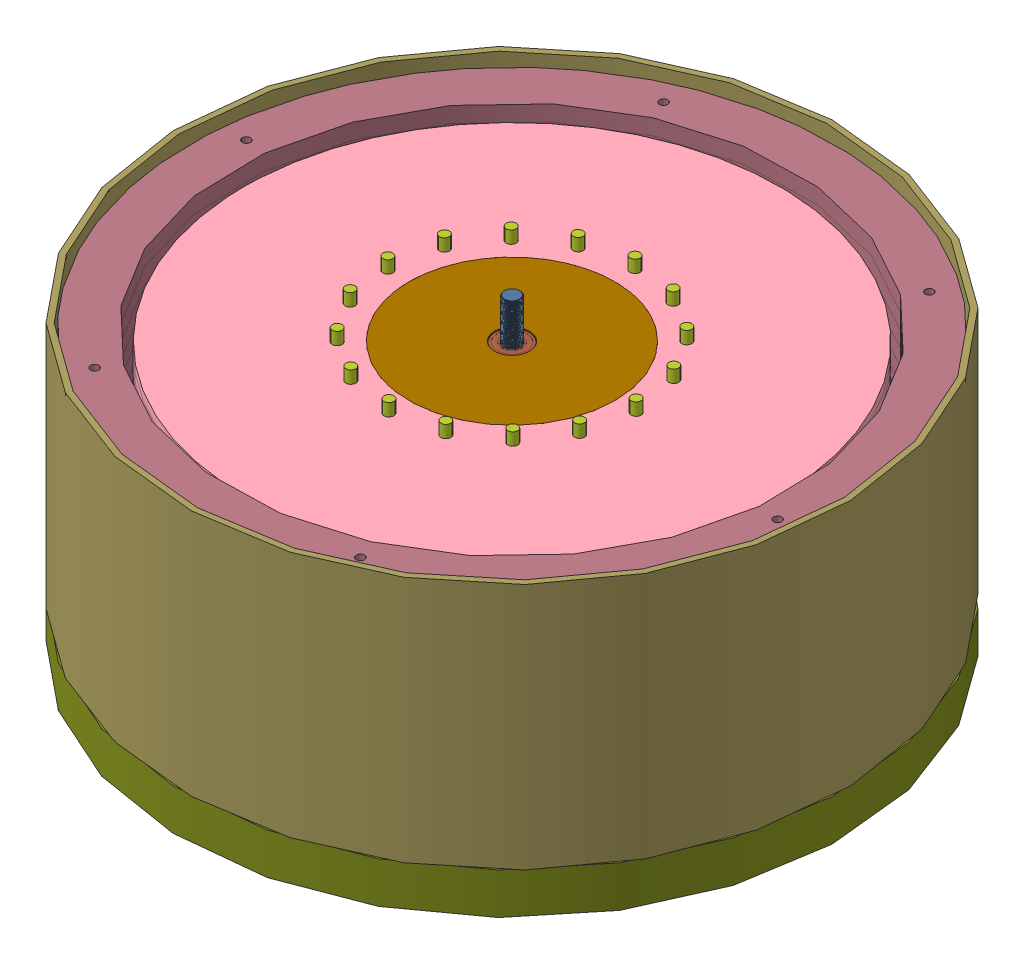
SolidWorks assembly Маховик 17, общая сборка, configuration Default. Lengths in mm.
Overall size (963.04 372.27 963.04).
101 component instances, 18 part files, 20 mates.
Components (placement in the parent):
- Маховик 17, сборка-1: Маховик 17, сборка [Default] at origin size (856.15 180 856.15)
  - Маховик 17, массив фланцев-1: Маховик 17, массив фланцев [Default] x (1 0 0) z (0 0 -1) size (652.89 50.1 652.89)
    - Маховик 17, сборка магнитов-1: Маховик 17, сборка магнитов [Default] x (-1 0 0) z (0 0 1) size (588.79 10.2 588.79)
      - Сегментный магнит-1: Сегментный магнит [Default] at (-0.1215 5 -242.8376) x (0.000409 0 1) z (-1 0 0.000409) size (102.7 10 114)
      - Магнит на Халбаха-1: Магнит на Халбаха [Default] at (-0.0877 0 0.2117) x (1 0 0) z (0 1 0) size (107.4 121.27 10.11)
      - Магнит на Халбаха 2-1: Магнит на Халбаха 2 [Default] at (0.1107 10 0.2672) x (-1 0 0) z (0 -1 0) size (107.4 121.27 10.11)
      - Сегментный магнит-43: Сегментный магнит [Default] at (171.692 5 -171.6691) x (-0.707396 0 0.706817) z (0.706817 0 0.707396) size (102.7 10 114)
      - Сегментный магнит-47: Сегментный магнит [Default] at (-242.8376 5 0.1215) x (1 0 -0.000409) z (0.000409 0 1) size (102.7 10 114)
      - Сегментный магнит-48: Сегментный магнит [Default] at (0.1215 5 242.8376) x (-0.000409 0 -1) z (1 0 -0.000409) size (102.7 10 114)
      - Сегментный магнит-49: Сегментный магнит [Default] at (242.8376 5 -0.1215) x (-1 0 0.000409) z (-0.000409 0 -1) size (102.7 10 114)
      - Сегментный магнит-50: Сегментный магнит [Default] at (-171.6691 5 -171.692) x (0.706817 0 0.707396) z (0.707396 0 -0.706817) size (102.7 10 114)
      - Сегментный магнит-51: Сегментный магнит [Default] at (-171.692 5 171.6691) x (0.707396 0 -0.706817) z (-0.706817 0 -0.707396) size (102.7 10 114)
      - Сегментный магнит-52: Сегментный магнит [Default] at (171.6691 5 171.692) x (-0.706817 0 -0.707396) z (-0.707396 0 0.706817) size (102.7 10 114)
      - Магнит на Халбаха-12: Магнит на Халбаха [Default] at (0.2117 0 0.0877) x (0 0 -1) z (0 1 0) size (107.4 121.27 10.11)
      - Магнит на Халбаха-13: Магнит на Халбаха [Default] at (0.0877 0 -0.2117) x (-1 0 0) z (0 1 0) size (107.4 121.27 10.11)
      - Магнит на Халбаха-14: Магнит на Халбаха [Default] at (-0.2117 0 -0.0877) x (0 0 1) z (0 1 0) size (107.4 121.27 10.11)
      - Магнит на Халбаха 2-5: Магнит на Халбаха 2 [Default] at (0.2672 10 -0.1107) x (0 0 1) z (0 -1 0) size (107.4 121.27 10.11)
      - Магнит на Халбаха 2-6: Магнит на Халбаха 2 [Default] at (-0.1107 10 -0.2672) x (1 0 0) z (0 -1 0) size (107.4 121.27 10.11)
      - Магнит на Халбаха 2-7: Магнит на Халбаха 2 [Default] at (-0.2672 10 0.1107) x (0 0 -1) z (0 -1 0) size (107.4 121.27 10.11)
    - Маховик 17, глухой фланец-1: Маховик 17, глухой фланец [Default] at (0.1668 -10 0.2735) x (-0.99999 0 -0.004449) z (0 -1 0) size (650 650 10)
    - Маховик 17, фланец под магниты-1: Маховик 17, фланец под магниты [Default] at (0.1668 0 0.2735) x (0.99999 0 0.004449) z (0 -1 0) size (650 650 10)
    - Маховик 17, глухой фланец-2: Маховик 17, глухой фланец [Default] at (0.1668 -20 0.2735) x (-0.99999 0 -0.004449) z (0 -1 0) size (650 650 10)
    - Маховик 17, глухой фланец-3: Маховик 17, глухой фланец [Default] at (0.1668 -30 0.2735) x (-0.99999 0 -0.004449) z (0 -1 0) size (650 650 10)
    - Маховик 17, глухой фланец-4: Маховик 17, глухой фланец [Default] at (0.1668 -40 0.2735) x (-0.99999 0 -0.004449) z (0 -1 0) size (650 650 10)
  - Маховик 17, массив фланцев-2: Маховик 17, массив фланцев [Default] at (0.3533 -50 -0.5339) x (0.390889 0 0.920438) z (-0.920438 0 0.390889) size (652.89 50.1 652.89)
    - Маховик 17, сборка магнитов-1: Маховик 17, сборка магнитов [Default] x (-1 0 0) z (0 0 1) size (588.79 10.2 588.79)
      - Сегментный магнит-1: Сегментный магнит [Default] at (-0.1215 5 -242.8376) x (0.000409 0 1) z (-1 0 0.000409) size (102.7 10 114)
      - Магнит на Халбаха-1: Магнит на Халбаха [Default] at (-0.0877 0 0.2117) x (1 0 0) z (0 1 0) size (107.4 121.27 10.11)
      - Магнит на Халбаха 2-1: Магнит на Халбаха 2 [Default] at (0.1107 10 0.2672) x (-1 0 0) z (0 -1 0) size (107.4 121.27 10.11)
      - Сегментный магнит-43: Сегментный магнит [Default] at (171.692 5 -171.6691) x (-0.707396 0 0.706817) z (0.706817 0 0.707396) size (102.7 10 114)
      - Сегментный магнит-47: Сегментный магнит [Default] at (-242.8376 5 0.1215) x (1 0 -0.000409) z (0.000409 0 1) size (102.7 10 114)
      - Сегментный магнит-48: Сегментный магнит [Default] at (0.1215 5 242.8376) x (-0.000409 0 -1) z (1 0 -0.000409) size (102.7 10 114)
      - Сегментный магнит-49: Сегментный магнит [Default] at (242.8376 5 -0.1215) x (-1 0 0.000409) z (-0.000409 0 -1) size (102.7 10 114)
      - Сегментный магнит-50: Сегментный магнит [Default] at (-171.6691 5 -171.692) x (0.706817 0 0.707396) z (0.707396 0 -0.706817) size (102.7 10 114)
      - Сегментный магнит-51: Сегментный магнит [Default] at (-171.692 5 171.6691) x (0.707396 0 -0.706817) z (-0.706817 0 -0.707396) size (102.7 10 114)
      - Сегментный магнит-52: Сегментный магнит [Default] at (171.6691 5 171.692) x (-0.706817 0 -0.707396) z (-0.707396 0 0.706817) size (102.7 10 114)
      - Магнит на Халбаха-12: Магнит на Халбаха [Default] at (0.2117 0 0.0877) x (0 0 -1) z (0 1 0) size (107.4 121.27 10.11)
      - Магнит на Халбаха-13: Магнит на Халбаха [Default] at (0.0877 0 -0.2117) x (-1 0 0) z (0 1 0) size (107.4 121.27 10.11)
      - Магнит на Халбаха-14: Магнит на Халбаха [Default] at (-0.2117 0 -0.0877) x (0 0 1) z (0 1 0) size (107.4 121.27 10.11)
      - Магнит на Халбаха 2-5: Магнит на Халбаха 2 [Default] at (0.2672 10 -0.1107) x (0 0 1) z (0 -1 0) size (107.4 121.27 10.11)
      - Магнит на Халбаха 2-6: Магнит на Халбаха 2 [Default] at (-0.1107 10 -0.2672) x (1 0 0) z (0 -1 0) size (107.4 121.27 10.11)
      - Магнит на Халбаха 2-7: Магнит на Халбаха 2 [Default] at (-0.2672 10 0.1107) x (0 0 -1) z (0 -1 0) size (107.4 121.27 10.11)
    - Маховик 17, глухой фланец-1: Маховик 17, глухой фланец [Default] at (0.1668 -10 0.2735) x (-0.99999 0 -0.004449) z (0 -1 0) size (650 650 10)
    - Маховик 17, фланец под магниты-1: Маховик 17, фланец под магниты [Default] at (0.1668 0 0.2735) x (0.99999 0 0.004449) z (0 -1 0) size (650 650 10)
    - Маховик 17, глухой фланец-2: Маховик 17, глухой фланец [Default] at (0.1668 -20 0.2735) x (-0.99999 0 -0.004449) z (0 -1 0) size (650 650 10)
    - Маховик 17, глухой фланец-3: Маховик 17, глухой фланец [Default] at (0.1668 -30 0.2735) x (-0.99999 0 -0.004449) z (0 -1 0) size (650 650 10)
    - Маховик 17, глухой фланец-4: Маховик 17, глухой фланец [Default] at (0.1668 -40 0.2735) x (-0.99999 0 -0.004449) z (0 -1 0) size (650 650 10)
  - Маховик 17, промежуточный фланец-1: Маховик 17, промежуточный фланец [Default] at (0.1668 -45 -0.2735) x (-0.004449 0 -0.99999) z (-0.99999 0 0.004449) size (350 10 350)
  - Маховик 17, промежуточный фланец-2: Маховик 17, промежуточный фланец [Default] at (0.1668 -35 -0.2735) x (-0.004449 0 -0.99999) z (-0.99999 0 0.004449) size (350 10 350)
  - Маховик 17, промежуточный фланец-3: Маховик 17, промежуточный фланец [Default] at (0.1668 -25 -0.2735) x (-0.004449 0 -0.99999) z (-0.99999 0 0.004449) size (350 10 350)
  - Маховик 17, промежуточный фланец-4: Маховик 17, промежуточный фланец [Default] at (0.1668 -15 -0.2735) x (-0.004449 0 -0.99999) z (-0.99999 0 0.004449) size (350 10 350)
  - Маховик 17, промежуточный фланец-5: Маховик 17, промежуточный фланец [Default] at (0.1668 -5 -0.2735) x (-0.004449 0 -0.99999) z (-0.99999 0 0.004449) size (350 10 350)
  - Маховик 17, фланец магнитной подушки-1: Маховик 17, фланец магнитной подушки [Default] at (0.1668 318.977 -0.2735) x (-0.556364 0.686266 0.468506) z (0.745396 0.661361 -0.08358) size (258 335.09 265.83) (hidden)
  - Шпилька М12-1: Шпилька М12 [Default] at (-149.8317 -25 0.3939) x (0.997876 0 0.065141) z (-0.065141 0 0.997876) size (12 180 12)
  - Шпилька М12-2: Шпилька М12 [Default] at (-138.1583 -25 57.745) x (0.946845 0 -0.321689) z (0.321689 0 0.946845) size (12 180 12)
  - Шпилька М12-3: Шпилька М12 [Default] at (-105.4263 -25 106.2634) x (0.751666 0 -0.659544) z (0.659544 0 0.751666) size (12 180 12)
  - Шпилька М12-4: Шпилька М12 [Default] at (-56.6186 -25 138.5625) x (0.442053 0 -0.896989) z (0.896989 0 0.442053) size (12 180 12)
  - Шпилька М12-5: Шпилька М12 [Default] at (0.8342 -25 149.725) x (0.065141 0 -0.997876) z (0.997876 0 0.065141) size (12 180 12)
  - Шпилька М12-6: Шпилька М12 [Default] at (58.1853 -25 138.0517) x (-0.321689 0 -0.946845) z (0.946845 0 -0.321689) size (12 180 12)
  - Шпилька М12-7: Шпилька М12 [Default] at (106.7037 -25 105.3196) x (-0.659544 0 -0.751666) z (0.751666 0 -0.659544) size (12 180 12)
  - Шпилька М12-8: Шпилька М12 [Default] at (139.0028 -25 56.5119) x (-0.896989 0 -0.442053) z (0.442053 0 -0.896989) size (12 180 12)
  - Шпилька М12-9: Шпилька М12 [Default] at (150.1654 -25 -0.9408) x (-0.997876 0 -0.065141) z (0.065141 0 -0.997876) size (12 180 12)
  - Шпилька М12-10: Шпилька М12 [Default] at (138.492 -25 -58.292) x (-0.946845 0 0.321689) z (-0.321689 0 -0.946845) size (12 180 12)
  - Шпилька М12-11: Шпилька М12 [Default] at (105.7599 -25 -106.8103) x (-0.751666 0 0.659544) z (-0.659544 0 -0.751666) size (12 180 12)
  - Шпилька М12-12: Шпилька М12 [Default] at (56.9522 -25 -139.1094) x (-0.442053 0 0.896989) z (-0.896989 0 -0.442053) size (12 180 12)
  - Шпилька М12-13: Шпилька М12 [Default] at (-0.5005 -25 -150.272) x (-0.065141 0 0.997876) z (-0.997876 0 -0.065141) size (12 180 12)
  - Шпилька М12-14: Шпилька М12 [Default] at (-57.8516 -25 -138.5987) x (0.321689 0 0.946845) z (-0.946845 0 0.321689) size (12 180 12)
  - Шпилька М12-15: Шпилька М12 [Default] at (-106.37 -25 -105.8666) x (0.659544 0 0.751666) z (-0.751666 0 0.659544) size (12 180 12)
  - Шпилька М12-16: Шпилька М12 [Default] at (-138.6691 -25 -57.0589) x (0.896989 0 0.442053) z (-0.442053 0 0.896989) size (12 180 12)
  - Маховик 17, катушка-1: Маховик 17, катушка [Default] at (-73.7115 -47.5 -238.8782) x (0.954234 0 -0.29906) z (0.29906 0 0.954234) size (243 45 143.72)
  - Маховик 17, катушка-2: Маховик 17, катушка [Default] at (-220.792 -47.5 -116.7527) x (0.463278 0 -0.886213) z (0.886213 0 0.463278) size (243 45 143.72)
  - Маховик 17, катушка-3: Маховик 17, катушка [Default] at (-238.4379 -47.5 73.6048) x (-0.29906 0 -0.954234) z (0.954234 0 -0.29906) size (243 45 143.72)
  - Маховик 17, катушка-4: Маховик 17, катушка [Default] at (-116.3124 -47.5 220.6854) x (-0.886213 0 -0.463278) z (0.463278 0 -0.886213) size (243 45 143.72)
  - Маховик 17, катушка-5: Маховик 17, катушка [Default] at (74.0451 -47.5 238.3313) x (-0.954234 0 0.29906) z (-0.29906 0 -0.954234) size (243 45 143.72)
  - Маховик 17, катушка-6: Маховик 17, катушка [Default] at (221.1257 -47.5 116.2057) x (-0.463278 0 0.886213) z (-0.886213 0 -0.463278) size (243 45 143.72)
  - Маховик 17, катушка-7: Маховик 17, катушка [Default] at (238.7716 -47.5 -74.1518) x (0.29906 0 0.954234) z (-0.954234 0 0.29906) size (243 45 143.72)
  - Маховик 17, катушка-8: Маховик 17, катушка [Default] at (116.646 -47.5 -221.2324) x (0.886213 0 0.463278) z (-0.463278 0 0.886213) size (243 45 143.72)
  - 123-1: 123 [Default] at (0.1668 -115 -0.2735) x (-0.840967 0 -0.541087) z (0.541087 0 -0.840967) size (100 20 100) (hidden)
- Маховик 17, втулка-1: Маховик 17, втулка [Default] at (0.1668 -30 -0.2735) x (0.99999 0 -0.004449) z (0.004449 0 0.99999) size (360 160 360)
- Прототип 16, вал-1: Прототип 16, вал [Default] at (0.1668 3.7012 -0.2735) x (-0.996978 0 -0.077688) z (-0.077688 0 0.996978) size (30 321.49 30)
- 7004-1: 7004 [Default] at (0.1668 49 -0.2735) x (0 -1 0) z (-0.944589 0 0.328255) size (12 42 42)
- 7004-2: 7004 [Default] at (0.1668 -97 -0.2735) x (0 -1 0) z (-0.996913 0 -0.07851) size (12 42 42)
- Маховик 17, камера-1: Маховик 17, камера [Default] at (0.1668 -72.9784 -0.2735) x (0.999604 0 -0.02814) z (0.02814 0 0.999604) size (800 300 800)
- Маховик 17, МДФ-1: Маховик 17, МДФ [Default] at (0.1668 52.5216 -0.2735) x (0.994451 0 0.105198) z (-0.105198 0 0.994451) size (785 19 785)
- Маховик 17, різьбова втулка-1: Маховик 17, різьбова втулка [Default] at (0.1668 -205.9784 -0.2735) x (0.988748 0 -0.149589) z (0.149589 0 0.988748) size (95 130.57 95)
- Маховик 17, МДФ-2: Маховик 17, МДФ [Default] at (0.1668 33.5216 -0.2735) x (0.994451 0 0.105198) z (-0.105198 0 0.994451) size (785 19 785)
- Маховик 17, МДФ-3: Маховик 17, МДФ [Default] at (0.1668 14.5216 -0.2735) x (0.994451 0 0.105198) z (-0.105198 0 0.994451) size (785 19 785)
- Маховик 17, МДФ-4: Маховик 17, МДФ [Default] at (0.1668 -4.4784 -0.2735) x (0.994451 0 0.105198) z (-0.105198 0 0.994451) size (785 19 785)
- Маховик 17, МДФ-5: Маховик 17, МДФ [Default] at (0.1668 -23.4784 -0.2735) x (0.994451 0 0.105198) z (-0.105198 0 0.994451) size (785 19 785)
- Маховик 17, МДФ-6: Маховик 17, МДФ [Default] at (0.1668 -42.4784 -0.2735) x (0.994451 0 0.105198) z (-0.105198 0 0.994451) size (785 19 785)
- Маховик 17, МДФ-7: Маховик 17, МДФ [Default] at (0.1668 -61.4784 -0.2735) x (0.994451 0 0.105198) z (-0.105198 0 0.994451) size (785 19 785)
- Маховик 17, МДФ-8: Маховик 17, МДФ [Default] at (0.1668 -80.4784 -0.2735) x (0.994451 0 0.105198) z (-0.105198 0 0.994451) size (785 19 785)
- Маховик 17, МДФ-9: Маховик 17, МДФ [Default] at (0.1668 -99.4784 -0.2735) x (0.994451 0 0.105198) z (-0.105198 0 0.994451) size (785 19 785)
- Маховик 17, МДФ-10: Маховик 17, МДФ [Default] at (0.1668 -118.4784 -0.2735) x (0.994451 0 0.105198) z (-0.105198 0 0.994451) size (785 19 785)
- Маховик 17, бетонная бобышка-2: Маховик 17, бетонная бобышка [Default] at (0.1668 -190.9784 -0.2735) x (0.999533 0 0.030542) z (-0.030542 0 0.999533) size (675 64 675)
- Маховик 17, МДФ-11: Маховик 17, МДФ [Default] at (0.1668 -137.4784 -0.2735) x (0.994451 0 0.105198) z (-0.105198 0 0.994451) size (785 19 785)
- Маховик 17, МДФ-12: Маховик 17, МДФ [Default] at (0.1668 -156.4784 -0.2735) x (0.994451 0 0.105198) z (-0.105198 0 0.994451) size (785 19 785)
- Маховик 17, МДФ-13: Маховик 17, МДФ [Default] at (0.1668 -175.4784 -0.2735) x (0.994451 0 0.105198) z (-0.105198 0 0.994451) size (785 19 785)
- Маховик 17, МДФ-14: Маховик 17, МДФ [Default] at (0.1668 -194.4784 -0.2735) x (0.994451 0 0.105198) z (-0.105198 0 0.994451) size (785 19 785)
- Маховик 17, МДФ-15: Маховик 17, МДФ [Default] at (0.1668 -213.4784 -0.2735) x (0.994451 0 0.105198) z (-0.105198 0 0.994451) size (785 19 785)
- Маховик 17, фундамент-1: Маховик 17, фундамент [Default] at (0.1668 -247.9784 -0.2735) x (0.973002 0 -0.230798) z (0.230798 0 0.973002) size (800 50.52 800)
Mates (geometry in assembly coordinates):
- Coincident1: coincident aligned: plane of Маховик 17, сборка-1 through (0 0 0) normal (0 0 1)
- Coincident2: coincident aligned: plane of Маховик 17, сборка-1 through (0 0 0) normal (0 1 0)
- Coincident3: coincident aligned: plane of Маховик 17, сборка-1 through (0 0 0) normal (1 0 0)
- Concentric1: concentric aligned: cylinder of Маховик 17, сборка-1/Маховик 17, массив фланцев-2/Маховик 17, глухой фланец-4 through (0.1668 -100 -0.2735) axis (0 1 0) radius 125; cylinder of Маховик 17, втулка-1 through (0.1668 50 -0.2735) axis (0 1 0) radius 125
- Concentric2: concentric anti-aligned: cylinder of Маховик 17, сборка-1/Шпилька М12-8 through (139.0028 65 56.5119) axis (0 -1 0) radius 6; cylinder of Маховик 17, втулка-1 through (139.0028 -110 56.5119) axis (0 1 0) radius 6.1
- Coincident4: coincident anti-aligned: plane of Маховик 17, сборка-1/Маховик 17, массив фланцев-2/Маховик 17, глухой фланец-4 through (0.1668 -100 -0.2735) normal (0 -1 0); plane of Маховик 17, втулка-1 through (0.1668 -100 -0.2735) normal (0 1 0)
- Concentric3: concentric aligned: cylinder of Маховик 17, сборка-1/Маховик 17, массив фланцев-1/Маховик 17, глухой фланец-3 through (0.1668 40 -0.2735) axis (0 -1 0) radius 325; cylinder of Прототип 16, вал-1 through (0.1668 -79.8282 -0.2735) axis (0 -1 0) radius 10
- Concentric4: concentric aligned: cylinder of Маховик 17, втулка-1 through (0.1668 50 -0.2735) axis (0 1 0) radius 21.25; cylinder of 7004-1 through (0.1668 43 -0.2735) axis (0 1 0) radius 10
- Coincident5: coincident anti-aligned: plane of Маховик 17, втулка-1 through (0.1668 37 -0.2735) normal (0 1 0); plane of 7004-1 through (-18.7013 37 6.2834) normal (0 -1 0)
- Concentric5: concentric anti-aligned: cylinder of Прототип 16, вал-1 through (0.1668 -79.8282 -0.2735) axis (0 -1 0) radius 10; cylinder of 7004-2 through (0.1668 -103 -0.2735) axis (0 1 0) radius 21
- Coincident6: coincident anti-aligned: plane of Маховик 17, втулка-1 through (0.1668 -97 -0.2735) normal (0 -1 0); plane of 7004-2 through (-18.949 -97 -1.7789) normal (0 1 0)
- Concentric6: concentric aligned: cylinder of Маховик 17, сборка-1/Маховик 17, массив фланцев-1/Маховик 17, фланец под магниты-1 through (0.1668 10 -0.2735) axis (0 -1 0) radius 325; cylinder of Маховик 17, камера-1 through (0.1668 77.0216 -0.2735) axis (0 -1 0) radius 400
- Concentric7: concentric anti-aligned: cylinder of Маховик 17, сборка-1/Маховик 17, массив фланцев-1/Маховик 17, фланец под магниты-1 through (0.1668 10 -0.2735) axis (0 -1 0) radius 325; cylinder of Маховик 17, різьбова втулка-1 through (0.1668 -122.0644 -0.2735) axis (0 1 0) radius 47.5
- Concentric8: concentric anti-aligned: cylinder of Маховик 17, сборка-1/Маховик 17, промежуточный фланец-2 through (0.1668 -40 -0.2735) axis (0 1 0) radius 175; cylinder of Маховик 17, МДФ-1 through (0.1668 62.0216 -0.2735) axis (0 -1 0) radius 337.5
- Concentric9: concentric aligned: cylinder of Маховик 17, камера-1 through (0.1668 77.0216 -0.2735) axis (0 -1 0) radius 400; cylinder of Маховик 17, бетонная бобышка-2 through (0.1668 -158.9784 -0.2735) axis (0 -1 0) radius 337.5
- Concentric10: concentric aligned: cylinder of Маховик 17, камера-1 through (0.1668 77.0216 -0.2735) axis (0 -1 0) radius 400; cylinder of Маховик 17, фундамент-1 through (0.1668 -222.9784 -0.2735) axis (0 -1 0) radius 400
- Coincident7: coincident anti-aligned: plane of Маховик 17, камера-1 through (0.1668 -222.9784 -0.2735) normal (0 -1 0); plane of Маховик 17, фундамент-1 through (0.1668 -222.9784 -0.2735) normal (0 1 0)
- Coincident8: coincident anti-aligned: plane of Маховик 17, бетонная бобышка-2 through (0.1668 -222.9784 -0.2735) normal (0 -1 0); plane of Маховик 17, фундамент-1 through (0.1668 -222.9784 -0.2735) normal (0 1 0)
- Coincident9: coincident anti-aligned: plane of Маховик 17, МДФ-15 through (0.1668 -222.9784 -0.2735) normal (0 -1 0); plane of Маховик 17, фундамент-1 through (0.1668 -222.9784 -0.2735) normal (0 1 0)
- Coincident10: coincident anti-aligned: plane of Маховик 17, різьбова втулка-1 through (0.1668 -262.9784 -0.2735) normal (0 -1 0); plane of Маховик 17, фундамент-1 through (0.1668 -262.9784 -0.2735) normal (0 1 0)
